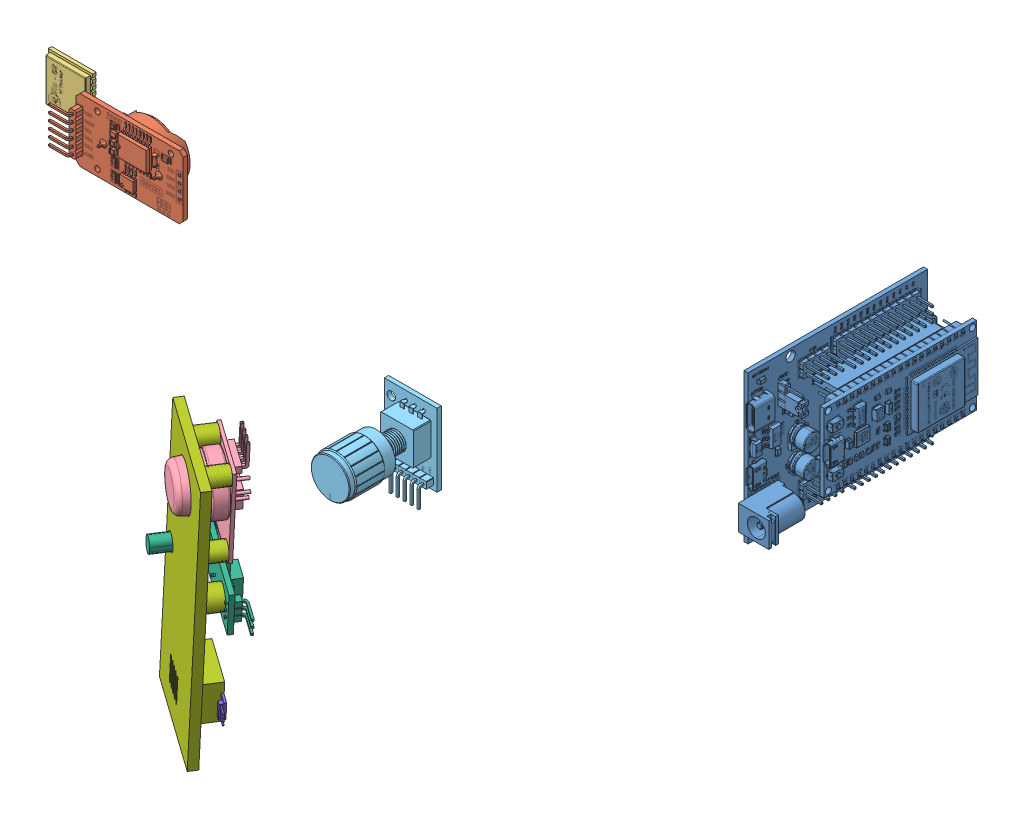
SolidWorks assembly assy_base1_1, configuration Default. Lengths in mm.
Overall size (279.39 180.91 128.1).
10 component instances, 8 part files, 10 mates.
Components (placement in the parent):
- ESP32_con_expansion-1: ESP32_con_expansion [Default] at (26.7569 179.9117 292.8512) x (0 1 0) z (0 0 -1) size (53.4 18.93 73.99)
- DS3231 RTC-1: DS3231 RTC [Default] at (-181.8049 170.5692 311.2869) size (44.75 22.8 13.53)
  - DS3231 RTC.step-1: DS3231 RTC.step [Default] at origin size (44.75 22.8 13.53)
    - Default.step-1: Default.step [Default] at origin size (44.75 22.8 13.53)
- LoRa_Module_RA-02_AiThinker-1: LoRa_Module_RA-02_AiThinker [Default] at (-205.1667 163.3039 300.0265) size (16 17 3.03)
- MQ135_sensor-1: MQ135_sensor [Default] at (-107.2364 120.9332 350.6426) x (0.138761 0.986168 0.090656) z (-0.546944 0 0.837169) size (36.7 20 20.1)
- Rotary Encoder - KY-040-1: Rotary Encoder - KY-040 [Default] at (-84.7972 130.541 306.9197) size (19 30.75 32.39)
- LDR-1: LDR [Default] at (-115.9886 91.706 346.1979) x (0.138761 0.986168 0.090656) z (0.546944 0 -0.837169) size (14.2 40.8 21.6)
- soporte_sensores-2: soporte_sensores [Default] at (-100.5786 134.7229 366.9373) x (-0.138761 -0.986168 -0.090656) z (0.825589 -0.165751 0.539379) size (100 11 35)
- AHT25-1: AHT25 [Default] at (-111.7412 48.0139 346.6244) x (0.138761 0.986168 0.090656) z (0.825589 -0.165751 0.539379) size (6 2 17.7)
Mates (geometry in assembly coordinates):
- Coincident3: coincident: plane of MQ135_sensor-1 through (-112.1241 119.3794 347.4493) normal (-0.546944 0 0.837169); circle of soporte_sensores-2
- Concentric1: concentric: cylinder of MQ135_sensor-1 through (-107.8054 104.823 350.2708) axis (0.546944 0 -0.837169) radius 1.5; cylinder of soporte_sensores-2 through (-111.0871 104.823 355.2938) axis (0.546944 0 -0.837169) radius 1.25
- Concentric3: concentric: cylinder of MQ135_sensor-1 through (-104.0589 131.4496 352.7185) axis (0.546944 0 -0.837169) radius 1.5; cylinder of soporte_sensores-2 through (-107.3405 131.4496 357.7415) axis (0.546944 0 -0.837169) radius 1.25
- Coincident4: coincident: plane of LDR-1 through (-115.9525 91.706 346.1426) normal (-0.546944 0 0.837169); plane of soporte_sensores-2 through (-108.7132 90.1921 350.8722) normal (0.546944 0 -0.837169)
- Parallel4: parallel: plane of soporte_sensores-2 through (-98.9378 134.7229 364.4258) normal (0.546944 0 -0.837169); plane of AHT25-1 through (-111.7412 48.0139 346.6244) normal (0.546944 0 -0.837169)
- Coincident8: coincident: plane of soporte_sensores-2 through (-119.2993 46.3988 341.5671) normal (-0.825589 0.165751 -0.539379); plane of AHT25-1 through (-119.0986 50.9352 342.6538) normal (0.825589 -0.165751 0.539379)
- Coincident9: coincident: plane of soporte_sensores-2 through (-94.9998 134.7229 358.3982) normal (0.546944 0 -0.837169); plane of AHT25-1 through (-112.1241 48.0139 347.2104) normal (-0.546944 0 0.837169)
- Coincident12: coincident: plane of soporte_sensores-2 through (-118.6823 53.8937 342.9258) normal (-0.138761 -0.986168 -0.090656); plane of AHT25-1 through (-115.6276 53.2804 344.9215) normal (0.138761 0.986168 0.090656)
- Concentric4: concentric: cylinder of LDR-1 through (-107.8381 90.1921 349.5327) axis (0.546944 0 -0.837169) radius 1.5; cylinder of soporte_sensores-2 through (-108.7132 90.1921 350.8722) axis (-0.546944 0 0.837169) radius 1.25
- Parallel8: parallel: plane of MQ135_sensor-1 through (-106.0883 101.9432 351.3926) normal (-0.138761 -0.986168 -0.090656); plane of LDR-1 through (-127.955 101.2548 338.3011) normal (0.138761 0.986168 0.090656)
